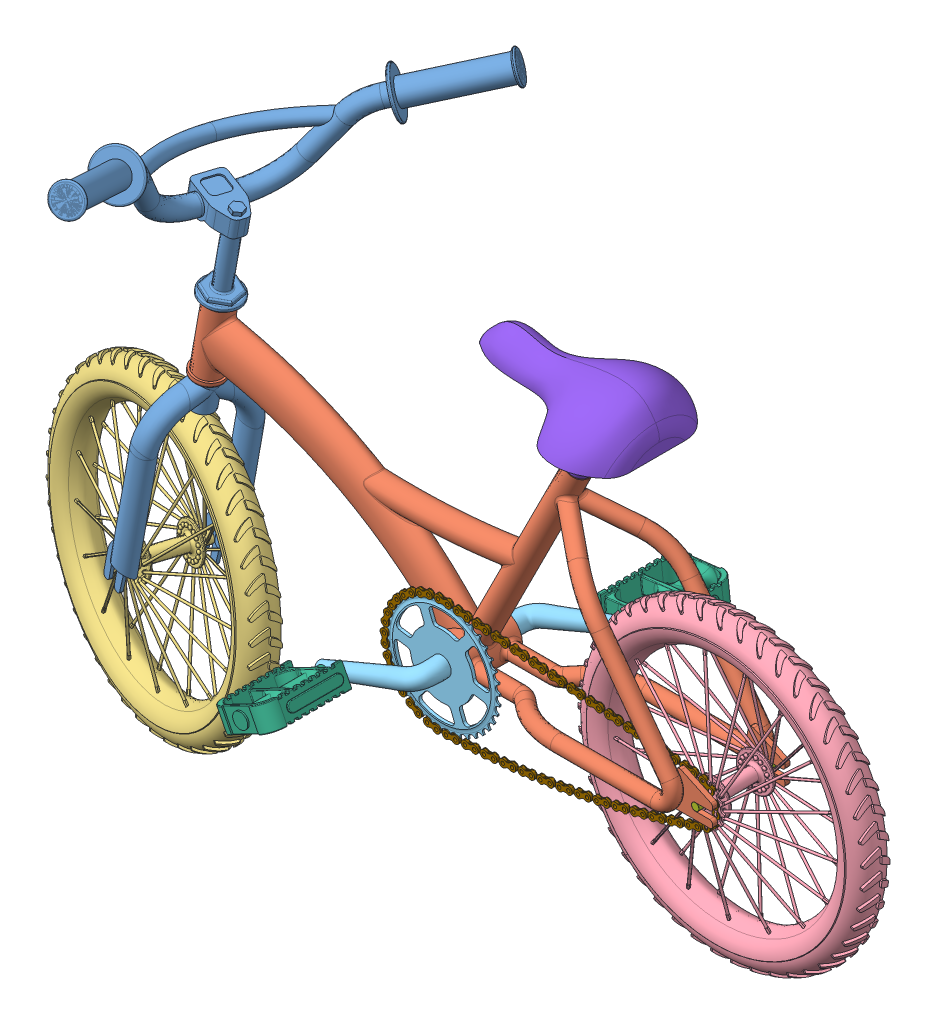
SolidWorks assembly rower, configuration Domyślna. Lengths in mm.
Overall size (1233.79 850.56 536.73).
12 component instances, 10 part files, 26 mates.
Components (placement in the parent):
- kierownica-1: kierownica [Domyślna] at (115.5847 135.1921 430.732) x (0.951481 -0.169753 0.256647) z (-0.252657 0.045076 0.966505) size (154.93 652.1 514.19)
- rama-1: rama [Domyślna] at (453.4879 -183.4977 435.865) size (736.48 311.09 139.06)
- koło_przednie-1: koło_przednie [Domyślna] at (41.2434 -280.9701 430.7074) x (0.252657 -0.045076 -0.966505) z (0.963953 -0.074392 0.25546) size (100 394.84 394.76)
- koło-1: koło [Domyślna] at (797.1977 -167.6577 435.865) x (0 0 -1) z (-0.922806 -0.385264 0) size (89 394.84 394.76)
- pedaly-1: pedaly [Domyślna] at (453.4879 -183.4977 434.865) x (0.93014 0.367206 0) z (0 0 -1) size (270.08 150.67 179.12)
- pedał-1: pedał [Domyślna] at (337.2204 -229.3984 576.865) x (0 0 1) z (0.452779 -0.891623 0) size (110.71 84 30.09)
- pedał-2: pedał [Domyślna] at (569.7554 -137.597 292.865) x (0 0 -1) z (-0.115308 0.99333 0) size (110.71 84 30.09)
- kołek-1: kołek [Domyślna] at (797.1977 -167.6577 435.865) x (-0.293797 -0.955868 0) z (0 0 1) size (10 10 102)
- kołek-2: kołek [Domyślna] at (41.2434 -280.9701 430.7074) x (0.316064 -0.94027 0.126476) z (-0.252657 0.045076 0.966505) size (10 10 102)
- siodelko-1: siodelko [Domyślna] at (585.0548 169.7975 435.865) x (0.993081 -0.117428 0) z (0 0 1) size (229.49 205.06 178.42)
- łańcuch-1: łańcuch [Domyślna] at (579.9892 -120.0751 476.365) x (-0.995598 0.093727 0) z (0 0 -1) size (444.64 160.52 4)
- radial ball bearing_68_am-2: radial ball bearing_68_am [AFBMA 20.1 - 42-25 - 12,SI,NC,12_68] at (453.4879 -183.4977 411.865) x (0 0 1) z (0.468111 -0.88367 0) size (27 52 52)
Mates (geometry in assembly coordinates):
- Koncentryczne1: concentric anti-aligned: cylinder of kierownica-1 through (122.4955 63.8696 435.865) axis (-0.175635 -0.984455 0) radius 15; circle of rama-1
- Wspólnie1: coincident anti-aligned: plane of kierownica-1 through (120.7391 54.0251 435.865) normal (-0.175635 -0.984455 0); plane of rama-1 through (120.7391 54.0251 435.865) normal (0.175635 0.984455 0)
- Koncentryczne2: concentric anti-aligned: cylinder of kierownica-1 through (27.5999 -278.536 482.8987) axis (0.252657 -0.045076 -0.966505) radius 5; cylinder of koło_przednie-1 through (50.9707 -282.7055 393.4969) axis (-0.252657 0.045076 0.966505) radius 8.8
- Szerokość1: width aligned: plane of kierownica-1 through (61.6648 -305.945 381.3392) normal (0.252657 -0.045076 -0.966505); plane of koło_przednie-1 through (34.3778 -301.0768 485.7218) normal (-0.252657 0.045076 0.966505); plane of kierownica-1 through (50.9707 -282.7055 393.4969) normal (0.252657 -0.045076 -0.966505); plane of koło_przednie-1 through (31.5161 -279.2346 467.9178) normal (-0.252657 0.045076 0.966505)
- Koncentryczne4: concentric aligned: cylinder of rama-1 through (797.1977 -167.6577 480.365) axis (0 0 1) radius 5; cylinder of koło-1 through (797.1977 -167.6577 397.365) axis (0 0 1) radius 8.8
- Szerokość3: width anti-aligned: plane of rama-1 through (797.1977 -167.6577 384.865) normal (0 0 -1); plane of rama-1 through (797.1977 -167.6577 486.865) normal (0 0 1); plane of koło-1 through (797.1977 -167.6577 480.365) normal (0 0 1); plane of koło-1 through (797.1977 -167.6577 391.365) normal (0 0 -1)
- Koncentryczne5: concentric aligned: cylinder of rama-1 through (453.4879 -183.4977 366.3346) axis (0 0 1) radius 26; cylinder of pedaly-1 through (453.4879 -183.4977 392.365) axis (0 0 1) radius 12.5
- Wspólnie2: coincident anti-aligned: plane of rama-1 through (453.4879 -183.4977 473.365) normal (0 0 1); plane of pedaly-1 through (486.2271 -164.7039 473.365) normal (0 0 -1)
- Koncentryczne6: concentric anti-aligned: cylinder of pedaly-1 through (515.7191 -291.9056 584.865) axis (0 0 -1) radius 5; cylinder of pedał-1 through (515.7191 -291.9056 526.865) axis (0 0 1) radius 7.5
- Wspólnie3: coincident anti-aligned: plane of pedaly-1 through (390.608 -375.2557 516.865) normal (0 0 1); plane of pedał-1 through (515.7191 -291.9056 516.865) normal (0 0 -1)
- Koncentryczne7: concentric aligned: cylinder of pedaly-1 through (391.2567 -75.0898 584.865) axis (0 0 -1) radius 5; cylinder of pedał-2 through (391.2567 -75.0898 342.865) axis (0 0 -1) radius 7.5
- Wspólnie4: coincident anti-aligned: plane of pedaly-1 through (256.1887 -141.0945 352.865) normal (0 0 -1); plane of pedał-2 through (391.2567 -75.0898 352.865) normal (0 0 1)
- Koncentryczne8: concentric anti-aligned: cylinder of koło_przednie-1 through (50.9707 -282.7055 393.4969) axis (-0.252657 0.045076 0.966505) radius 5; cylinder of kołek-2 through (28.3578 -278.6712 479.9991) axis (0.252657 -0.045076 -0.966505) radius 5
- Szerokość4: width anti-aligned: plane of kierownica-1 through (34.3778 -301.0768 485.7218) normal (-0.252657 0.045076 0.966505); plane of kierownica-1 through (61.6648 -305.945 381.3392) normal (0.252657 -0.045076 -0.966505); plane of kołek-2 through (54.1289 -283.269 381.4156) normal (0.252657 -0.045076 -0.966505); plane of kołek-2 through (28.3578 -278.6712 479.9991) normal (-0.252657 0.045076 0.966505)
- Koncentryczne9: concentric anti-aligned: cylinder of koło-1 through (797.1977 -167.6577 397.365) axis (0 0 1) radius 5; cylinder of kołek-1 through (797.1977 -167.6577 486.865) axis (0 0 -1) radius 5
- Szerokość5: width aligned: plane of rama-1 through (797.1977 -167.6577 384.865) normal (0 0 -1); plane of rama-1 through (797.1977 -167.6577 486.865) normal (0 0 1); plane of kołek-1 through (797.1977 -167.6577 384.865) normal (0 0 -1); plane of kołek-1 through (797.1977 -167.6577 486.865) normal (0 0 1)
- Koncentryczne10: concentric aligned: cylinder of rama-1 through (368.187 -352.778 435.865) axis (0.45 0.893029 0) radius 13.5; cylinder of siodelko-1 through (561.4879 30.8291 435.865) axis (0.45 0.893029 0) radius 14
- Odległość1: distance = 90 mm anti-aligned: plane of siodelko-1 through (606.2719 187.428 400.865) normal (-0.45 -0.893029 0); plane of rama-1 through (592.9879 93.3411 435.865) normal (0.45 0.893029 0)
- Równolegle1: parallel aligned: plane of siodelko-1 through (585.0548 169.7975 435.865) normal (0 0 1)
- Koncentryczne13: concentric aligned: circle of łańcuch-1; circle of pedaly-1
- Wspólnie7: coincident aligned: plane of koło-1 through (797.1977 -167.6577 478.365) normal (0 0 1); plane of łańcuch-1 through (819.0071 -162.6199 478.365) normal (0 0 1)
- Kąt1: planar angle = 0.093865 rad aligned: line of łańcuch-1 through (460.5174 -108.8279 476.365) axis (0.995598 -0.093727 0); axis of rama-1 through (624.8849 -175.9977 495.3944) axis (1 0 0)
- Koncentryczne21: concentric aligned: cylinder of pedaly-1 through (453.4879 -183.4977 392.365) axis (0 0 1) radius 12.5; cylinder of radial ball bearing_68_am-2 through (453.4879 -183.4977 391.2275) axis (0 0 1) radius 12.5
- Wspólnie10: coincident aligned: plane of rama-1 through (453.4879 -183.4977 398.365) normal (0 0 -1); plane of radial ball bearing_68_am-2 through (434.0913 -193.7727 398.365) normal (0 0 -1)
- Wiązanie kół zębatych1: gear = 303.0539 : 138.7178 mm: circle of pedaly-1; circle of koło-1
- Wiązanie kół zębatych2: gear = 303.0539 : 303.0539 mm: circle of koło-1; circle of koło_przednie-1
